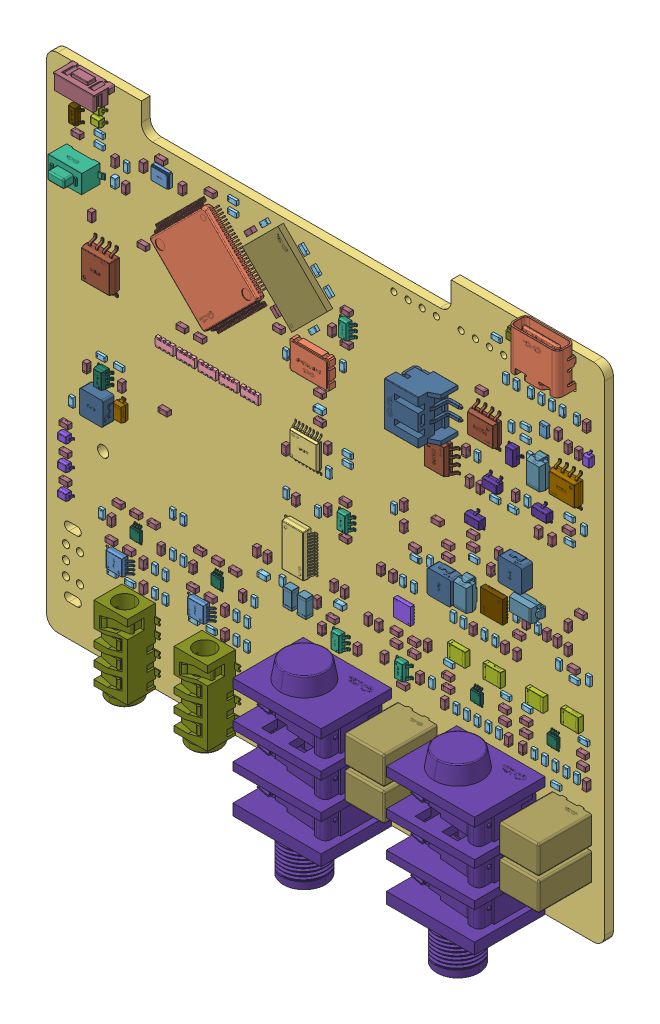
SolidWorks assembly 3D_board_2024-11-06, configuration 默认. Lengths in mm. (continued)
Components (placement in the parent): (continued)
- 3D_board_2024-11-06.step-1: 3D_board_2024-11-06.step [默认] at origin size (99.97 100.01 16.2) (continued)
  - iqks-C60.step-1: iqks-C60.step [默认] at (54.2011 -13.843 1.5862) x (-1 0 0) z (0 0 1) size (1.6 0.8 0.8) (continued)
    - C0603.step-1: C0603.step [默认] at origin size (1.6 0.8 0.8)
      - SOLID-10.step-1: SOLID-10.step [默认] at origin size (1.6 0.8 0.8)
  - iqks-C64.step-1: iqks-C64.step [默认] at (64.3026 -66.7617 1.5862) size (1.6 0.8 0.8)
    - C0603.step-1: C0603.step [默认] at origin size (1.6 0.8 0.8)
      - SOLID-10.step-1: SOLID-10.step [默认] at origin size (1.6 0.8 0.8)
  - iqks-C150.step-1: iqks-C150.step [默认] at (51.6811 -62.7701 1.5862) size (1.6 0.8 0.8)
    - C0603.step-1: C0603.step [默认] at origin size (1.6 0.8 0.8)
      - SOLID-10.step-1: SOLID-10.step [默认] at origin size (1.6 0.8 0.8)
  - iqks-C153.step-1: iqks-C153.step [默认] at (80.0102 -41.0211 1.5862) x (0 -1 0) z (0 0 1) size (1.6 0.8 0.8)
    - C0603.step-1: C0603.step [默认] at origin size (1.6 0.8 0.8)
      - SOLID-10.step-1: SOLID-10.step [默认] at origin size (1.6 0.8 0.8)
  - iqks-C15.step-1: iqks-C15.step [默认] at (71.7551 -65.8101 1.5862) x (0 1 0) z (0 0 1) size (1.6 0.8 0.8)
    - C0603.step-1: C0603.step [默认] at origin size (1.6 0.8 0.8)
      - SOLID-10.step-1: SOLID-10.step [默认] at origin size (1.6 0.8 0.8)
  - iqks-C16.step-1: iqks-C16.step [默认] at (83.1852 -65.8101 1.5862) x (0 1 0) z (0 0 1) size (1.6 0.8 0.8)
    - C0603.step-1: C0603.step [默认] at origin size (1.6 0.8 0.8)
      - SOLID-10.step-1: SOLID-10.step [默认] at origin size (1.6 0.8 0.8)
  - iqks-C38.step-1: iqks-C38.step [默认] at (85.7252 -65.8101 1.5862) x (0 1 0) z (0 0 1) size (1.6 0.8 0.8)
    - C0603.step-1: C0603.step [默认] at origin size (1.6 0.8 0.8)
      - SOLID-10.step-1: SOLID-10.step [默认] at origin size (1.6 0.8 0.8)
  - iqks-C39.step-1: iqks-C39.step [默认] at (97.1552 -65.8101 1.5862) x (0 1 0) z (0 0 1) size (1.6 0.8 0.8)
    - C0603.step-1: C0603.step [默认] at origin size (1.6 0.8 0.8)
      - SOLID-10.step-1: SOLID-10.step [默认] at origin size (1.6 0.8 0.8)
  - iqks-C17.step-1: iqks-C17.step [默认] at (26.6701 -67.3101 1.5862) x (0 -1 0) z (0 0 1) size (1.6 0.8 0.8)
    - C0603.step-1: C0603.step [默认] at origin size (1.6 0.8 0.8)
      - SOLID-10.step-1: SOLID-10.step [默认] at origin size (1.6 0.8 0.8)
  - iqks-C18.step-1: iqks-C18.step [默认] at (35.5601 -67.3101 1.5862) x (0 -1 0) z (0 0 1) size (1.6 0.8 0.8)
    - C0603.step-1: C0603.step [默认] at origin size (1.6 0.8 0.8)
      - SOLID-10.step-1: SOLID-10.step [默认] at origin size (1.6 0.8 0.8)
  - iqks-C50.step-1: iqks-C50.step [默认] at (12.065 -67.3101 1.5862) x (0 -1 0) z (0 0 1) size (1.6 0.8 0.8)
    - C0603.step-1: C0603.step [默认] at origin size (1.6 0.8 0.8)
      - SOLID-10.step-1: SOLID-10.step [默认] at origin size (1.6 0.8 0.8)
  - iqks-C51.step-1: iqks-C51.step [默认] at (20.955 -67.3101 1.5862) x (0 -1 0) z (0 0 1) size (1.6 0.8 0.8)
    - C0603.step-1: C0603.step [默认] at origin size (1.6 0.8 0.8)
      - SOLID-10.step-1: SOLID-10.step [默认] at origin size (1.6 0.8 0.8)
  - iqks-C22.step-1: iqks-C22.step [默认] at (17.78 -74.9301 1.5862) x (0 1 0) z (0 0 1) size (1.6 0.8 0.8)
    - C0603.step-1: C0603.step [默认] at origin size (1.6 0.8 0.8)
      - SOLID-10.step-1: SOLID-10.step [默认] at origin size (1.6 0.8 0.8)
  - iqks-C28.step-1: iqks-C28.step [默认] at (17.78 -71.1201 1.5862) x (0 -1 0) z (0 0 1) size (1.6 0.8 0.8)
    - C0603.step-1: C0603.step [默认] at origin size (1.6 0.8 0.8)
      - SOLID-10.step-1: SOLID-10.step [默认] at origin size (1.6 0.8 0.8)
  - iqks-C31.step-1: iqks-C31.step [默认] at (32.3851 -74.9301 1.5862) x (0 1 0) z (0 0 1) size (1.6 0.8 0.8)
    - C0603.step-1: C0603.step [默认] at origin size (1.6 0.8 0.8)
      - SOLID-10.step-1: SOLID-10.step [默认] at origin size (1.6 0.8 0.8)
  - iqks-C32.step-1: iqks-C32.step [默认] at (32.3851 -71.1201 1.5862) x (0 -1 0) z (0 0 1) size (1.6 0.8 0.8)
    - C0603.step-1: C0603.step [默认] at origin size (1.6 0.8 0.8)
      - SOLID-10.step-1: SOLID-10.step [默认] at origin size (1.6 0.8 0.8)
  - iqks-C113.step-1: iqks-C113.step [默认] at (53.8401 -57.5551 1.5862) x (0 1 0) z (0 0 1) size (1.6 0.8 0.8)
    - C0603.step-1: C0603.step [默认] at origin size (1.6 0.8 0.8)
      - SOLID-10.step-1: SOLID-10.step [默认] at origin size (1.6 0.8 0.8)
  - iqks-C116.step-1: iqks-C116.step [默认] at (38.1001 -59.0551 1.5862) x (0 1 0) z (0 0 1) size (1.6 0.8 0.8)
    - C0603.step-1: C0603.step [默认] at origin size (1.6 0.8 0.8)
      - SOLID-10.step-1: SOLID-10.step [默认] at origin size (1.6 0.8 0.8)
  - iqks-C25.step-1: iqks-C25.step [默认] at (63.1191 -60.9601 1.5862) x (-1 0 0) z (0 0 1) size (1.6 0.8 0.8)
    - C0603.step-1: C0603.step [默认] at origin size (1.6 0.8 0.8)
      - SOLID-10.step-1: SOLID-10.step [默认] at origin size (1.6 0.8 0.8)
  - iqks-C27.step-1: iqks-C27.step [默认] at (66.2941 -60.9601 1.5862) x (-1 0 0) z (0 0 1) size (1.6 0.8 0.8)
    - C0603.step-1: C0603.step [默认] at origin size (1.6 0.8 0.8)
      - SOLID-10.step-1: SOLID-10.step [默认] at origin size (1.6 0.8 0.8)
  - iqks-C129.step-1: iqks-C129.step [默认] at (58.0391 -59.6901 1.5862) x (0 1 0) z (0 0 1) size (1.6 0.8 0.8)
    - C0603.step-1: C0603.step [默认] at origin size (1.6 0.8 0.8)
      - SOLID-10.step-1: SOLID-10.step [默认] at origin size (1.6 0.8 0.8)
  - iqks-C154.step-1: iqks-C154.step [默认] at (60.3251 -50.8001 1.5862) x (0 -1 0) z (0 0 1) size (1.6 0.8 0.8)
    - C0603.step-1: C0603.step [默认] at origin size (1.6 0.8 0.8)
      - SOLID-10.step-1: SOLID-10.step [默认] at origin size (1.6 0.8 0.8)
  - iqks-C138.step-1: iqks-C138.step [默认] at (85.0902 -48.6411 1.5862) size (1.6 0.8 0.8)
    - C0603.step-1: C0603.step [默认] at origin size (1.6 0.8 0.8)
      - SOLID-10.step-1: SOLID-10.step [默认] at origin size (1.6 0.8 0.8)
  - iqks-C139.step-1: iqks-C139.step [默认] at (84.7092 -51.8161 1.5862) x (0 1 0) z (0 0 1) size (1.6 0.8 0.8)
    - C0603.step-1: C0603.step [默认] at origin size (1.6 0.8 0.8)
      - SOLID-10.step-1: SOLID-10.step [默认] at origin size (1.6 0.8 0.8)
  - iqks-C149.step-1: iqks-C149.step [默认] at (82.5502 -51.8161 1.5862) x (0 1 0) z (0 0 1) size (1.6 0.8 0.8)
    - C0603.step-1: C0603.step [默认] at origin size (1.6 0.8 0.8)
      - SOLID-10.step-1: SOLID-10.step [默认] at origin size (1.6 0.8 0.8)
  - iqks-C3.step-1: iqks-C3.step [默认] at (16.51 -64.1351 1.5862) x (-1 0 0) z (0 0 1) size (1.6 0.8 0.8)
    - C0603.step-1: C0603.step [默认] at origin size (1.6 0.8 0.8)
      - SOLID-10.step-1: SOLID-10.step [默认] at origin size (1.6 0.8 0.8)
  - iqks-C4.step-1: iqks-C4.step [默认] at (19.62 -64.1351 1.5862) size (1.6 0.8 0.8)
    - C0603.step-1: C0603.step [默认] at origin size (1.6 0.8 0.8)
      - SOLID-10.step-1: SOLID-10.step [默认] at origin size (1.6 0.8 0.8)
  - iqks-C5.step-1: iqks-C5.step [默认] at (13.335 -64.1351 1.5862) size (1.6 0.8 0.8)
    - C0603.step-1: C0603.step [默认] at origin size (1.6 0.8 0.8)
      - SOLID-10.step-1: SOLID-10.step [默认] at origin size (1.6 0.8 0.8)
  - iqks-C19.step-1: iqks-C19.step [默认] at (31.1151 -64.1351 1.5862) x (-1 0 0) z (0 0 1) size (1.6 0.8 0.8)
    - C0603.step-1: C0603.step [默认] at origin size (1.6 0.8 0.8)
      - SOLID-10.step-1: SOLID-10.step [默认] at origin size (1.6 0.8 0.8)
  - iqks-C20.step-1: iqks-C20.step [默认] at (34.225 -64.1351 1.5862) size (1.6 0.8 0.8)
    - C0603.step-1: C0603.step [默认] at origin size (1.6 0.8 0.8)
      - SOLID-10.step-1: SOLID-10.step [默认] at origin size (1.6 0.8 0.8)
  - iqks-C21.step-1: iqks-C21.step [默认] at (27.9401 -64.1351 1.5862) size (1.6 0.8 0.8)
    - C0603.step-1: C0603.step [默认] at origin size (1.6 0.8 0.8)
      - SOLID-10.step-1: SOLID-10.step [默认] at origin size (1.6 0.8 0.8)
  - iqks-C29.step-1: iqks-C29.step [默认] at (12.065 -70.4851 1.5862) size (1.6 0.8 0.8)
    - C0603.step-1: C0603.step [默认] at origin size (1.6 0.8 0.8)
      - SOLID-10.step-1: SOLID-10.step [默认] at origin size (1.6 0.8 0.8)
  - iqks-C30.step-1: iqks-C30.step [默认] at (15.24 -70.4851 1.5862) x (-1 0 0) z (0 0 1) size (1.6 0.8 0.8)
    - C0603.step-1: C0603.step [默认] at origin size (1.6 0.8 0.8)
      - SOLID-10.step-1: SOLID-10.step [默认] at origin size (1.6 0.8 0.8)
  - iqks-C33.step-1: iqks-C33.step [默认] at (26.6701 -70.4851 1.5862) size (1.6 0.8 0.8)
    - C0603.step-1: C0603.step [默认] at origin size (1.6 0.8 0.8)
      - SOLID-10.step-1: SOLID-10.step [默认] at origin size (1.6 0.8 0.8)
  - iqks-C36.step-1: iqks-C36.step [默认] at (29.8451 -70.4851 1.5862) x (-1 0 0) z (0 0 1) size (1.6 0.8 0.8)
    - C0603.step-1: C0603.step [默认] at origin size (1.6 0.8 0.8)
      - SOLID-10.step-1: SOLID-10.step [默认] at origin size (1.6 0.8 0.8)
  - iqks-C42.step-1: iqks-C42.step [默认] at (76.2002 -29.2101 1.5862) x (0 1 0) z (0 0 1) size (1.6 0.8 0.8)
    - C0603.step-1: C0603.step [默认] at origin size (1.6 0.8 0.8)
      - SOLID-10.step-1: SOLID-10.step [默认] at origin size (1.6 0.8 0.8)
  - iqks-C43.step-1: iqks-C43.step [默认] at (92.0752 -13.97 1.5862) x (0 1 0) z (0 0 1) size (1.6 0.8 0.8)
    - C0603.step-1: C0603.step [默认] at origin size (1.6 0.8 0.8)
      - SOLID-10.step-1: SOLID-10.step [默认] at origin size (1.6 0.8 0.8)
  - iqks-C44.step-1: iqks-C44.step [默认] at (93.8532 -15.113 1.5862) x (0 -1 0) z (0 0 1) size (1.6 0.8 0.8)
    - C0603.step-1: C0603.step [默认] at origin size (1.6 0.8 0.8)
      - SOLID-10.step-1: SOLID-10.step [默认] at origin size (1.6 0.8 0.8)
  - iqks-C46.step-1: iqks-C46.step [默认] at (78.1052 -29.2101 1.5862) x (0 1 0) z (0 0 1) size (1.6 0.8 0.8)
    - C0603.step-1: C0603.step [默认] at origin size (1.6 0.8 0.8)
      - SOLID-10.step-1: SOLID-10.step [默认] at origin size (1.6 0.8 0.8)
  - iqks-C49.step-1: iqks-C49.step [默认] at (93.9802 -27.9401 1.5862) x (-1 0 0) z (0 0 1) size (1.6 0.8 0.8)
    - C0603.step-1: C0603.step [默认] at origin size (1.6 0.8 0.8)
      - SOLID-10.step-1: SOLID-10.step [默认] at origin size (1.6 0.8 0.8)
  - iqks-C54.step-1: iqks-C54.step [默认] at (81.4072 -37.8461 1.5862) x (0 1 0) z (0 0 1) size (1.6 0.8 0.8)
    - C0603.step-1: C0603.step [默认] at origin size (1.6 0.8 0.8)
      - SOLID-10.step-1: SOLID-10.step [默认] at origin size (1.6 0.8 0.8)
  - iqks-C56.step-1: iqks-C56.step [默认] at (76.8352 -37.2111 1.5862) x (-1 0 0) z (0 0 1) size (1.6 0.8 0.8)
    - C0603.step-1: C0603.step [默认] at origin size (1.6 0.8 0.8)
      - SOLID-10.step-1: SOLID-10.step [默认] at origin size (1.6 0.8 0.8)
  - iqks-C61.step-1: iqks-C61.step [默认] at (56.1101 -65.3101 1.5862) x (0 1 0) z (0 0 1) size (1.6 0.8 0.8)
    - C0603.step-1: C0603.step [默认] at origin size (1.6 0.8 0.8)
      - SOLID-10.step-1: SOLID-10.step [默认] at origin size (1.6 0.8 0.8)
  - iqks-C134.step-1: iqks-C134.step [默认] at (75.5652 -24.765 1.5862) x (0 -1 0) z (0 0 1) size (1.6 0.8 0.8)
    - C0603.step-1: C0603.step [默认] at origin size (1.6 0.8 0.8)
      - SOLID-10.step-1: SOLID-10.step [默认] at origin size (1.6 0.8 0.8)
  - iqks-C135.step-1: iqks-C135.step [默认] at (84.4552 -27.3051 1.5862) x (0 -1 0) z (0 0 1) size (1.6 0.8 0.8)
    - C0603.step-1: C0603.step [默认] at origin size (1.6 0.8 0.8)
      - SOLID-10.step-1: SOLID-10.step [默认] at origin size (1.6 0.8 0.8)
  - iqks-C140.step-1: iqks-C140.step [默认] at (72.3901 -42.9261 1.5862) x (-1 0 0) z (0 0 1) size (1.6 0.8 0.8)
    - C0603.step-1: C0603.step [默认] at origin size (1.6 0.8 0.8)
      - SOLID-10.step-1: SOLID-10.step [默认] at origin size (1.6 0.8 0.8)
  - iqks-C141.step-1: iqks-C141.step [默认] at (72.3901 -41.0211 1.5862) x (-1 0 0) z (0 0 1) size (1.6 0.8 0.8)
    - C0603.step-1: C0603.step [默认] at origin size (1.6 0.8 0.8)
      - SOLID-10.step-1: SOLID-10.step [默认] at origin size (1.6 0.8 0.8)
  - iqks-C146.step-1: iqks-C146.step [默认] at (90.0432 -46.1011 1.5862) x (0 -1 0) z (0 0 1) size (1.6 0.8 0.8)
    - C0603.step-1: C0603.step [默认] at origin size (1.6 0.8 0.8)
      - SOLID-10.step-1: SOLID-10.step [默认] at origin size (1.6 0.8 0.8)
  - iqks-C147.step-1: iqks-C147.step [默认] at (91.9482 -46.1011 1.5862) x (0 1 0) z (0 0 1) size (1.6 0.8 0.8)
    - C0603.step-1: C0603.step [默认] at origin size (1.6 0.8 0.8)
      - SOLID-10.step-1: SOLID-10.step [默认] at origin size (1.6 0.8 0.8)
  - iqks-C151.step-1: iqks-C151.step [默认] at (49.7601 -65.3101 1.5862) x (0 -1 0) z (0 0 1) size (1.6 0.8 0.8)
    - C0603.step-1: C0603.step [默认] at origin size (1.6 0.8 0.8)
      - SOLID-10.step-1: SOLID-10.step [默认] at origin size (1.6 0.8 0.8)
  - iqks-C156.step-1: iqks-C156.step [默认] at (64.4229 -42.0779 1.5862) x (0 -1 0) z (0 0 1) size (1.6 0.8 0.8)
    - C0603.step-1: C0603.step [默认] at origin size (1.6 0.8 0.8)
      - SOLID-10.step-1: SOLID-10.step [默认] at origin size (1.6 0.8 0.8)
  - iqks-C159.step-1: iqks-C159.step [默认] at (93.8532 -46.4821 1.5862) x (0 -1 0) z (0 0 1) size (1.6 0.8 0.8)
    - C0603.step-1: C0603.step [默认] at origin size (1.6 0.8 0.8)
      - SOLID-10.step-1: SOLID-10.step [默认] at origin size (1.6 0.8 0.8)
  - iqks-C162.step-1: iqks-C162.step [默认] at (93.8532 -42.7991 1.5862) x (0 -1 0) z (0 0 1) size (1.6 0.8 0.8)
    - C0603.step-1: C0603.step [默认] at origin size (1.6 0.8 0.8)
      - SOLID-10.step-1: SOLID-10.step [默认] at origin size (1.6 0.8 0.8)
  - iqks-C163.step-1: iqks-C163.step [默认] at (64.4229 -38.7759 1.5862) x (0 -1 0) z (0 0 1) size (1.6 0.8 0.8)
    - C0603.step-1: C0603.step [默认] at origin size (1.6 0.8 0.8)
      - SOLID-10.step-1: SOLID-10.step [默认] at origin size (1.6 0.8 0.8)
  - iqks-C1.step-1: iqks-C1.step [默认] at (54.2011 -18.923 1.5862) size (1.6 0.8 0.8)
    - C0603.step-1: C0603.step [默认] at origin size (1.6 0.8 0.8)
      - SOLID-10.step-1: SOLID-10.step [默认] at origin size (1.6 0.8 0.8)
  - iqks-C2.step-1: iqks-C2.step [默认] at (51.5621 -18.0991 1.5862) x (0 1 0) z (0 0 1) size (1.6 0.8 0.8)
    - C0603.step-1: C0603.step [默认] at origin size (1.6 0.8 0.8)
      - SOLID-10.step-1: SOLID-10.step [默认] at origin size (1.6 0.8 0.8)
  - iqks-C57.step-1: iqks-C57.step [默认] at (86.3602 -46.1011 1.5862) x (0 -1 0) z (0 0 1) size (1.6 0.8 0.8)
    - C0603.step-1: C0603.step [默认] at origin size (1.6 0.8 0.8)
      - SOLID-10.step-1: SOLID-10.step [默认] at origin size (1.6 0.8 0.8)
  - iqks-C94.step-1: iqks-C94.step [默认] at (53.9751 -49.1491 1.5862) size (1.6 0.8 0.8)
    - C0603.step-1: C0603.step [默认] at origin size (1.6 0.8 0.8)
      - SOLID-10.step-1: SOLID-10.step [默认] at origin size (1.6 0.8 0.8)
  - iqks-C95.step-1: iqks-C95.step [默认] at (50.8001 -46.3551 1.5862) x (0 -1 0) z (0 0 1) size (1.6 0.8 0.8)
    - C0603.step-1: C0603.step [默认] at origin size (1.6 0.8 0.8)
      - SOLID-10.step-1: SOLID-10.step [默认] at origin size (1.6 0.8 0.8)
  - iqks-C96.step-1: iqks-C96.step [默认] at (60.9601 -64.1351 1.5862) x (0 1 0) z (0 0 1) size (1.6 0.8 0.8)
    - C0603.step-1: C0603.step [默认] at origin size (1.6 0.8 0.8)
      - SOLID-10.step-1: SOLID-10.step [默认] at origin size (1.6 0.8 0.8)
  - iqks-C97.step-1: iqks-C97.step [默认] at (67.3101 -64.1351 1.5862) x (0 1 0) z (0 0 1) size (1.6 0.8 0.8)
    - C0603.step-1: C0603.step [默认] at origin size (1.6 0.8 0.8)
      - SOLID-10.step-1: SOLID-10.step [默认] at origin size (1.6 0.8 0.8)
  - iqks-C148.step-1: iqks-C148.step [默认] at (76.8352 -51.8161 1.5862) x (0 -1 0) z (0 0 1) size (1.6 0.8 0.8)
    - C0603.step-1: C0603.step [默认] at origin size (1.6 0.8 0.8)
      - SOLID-10.step-1: SOLID-10.step [默认] at origin size (1.6 0.8 0.8)
  - iqks-C164.step-1: iqks-C164.step [默认] at (66.4211 -44.4501 1.5862) x (-1 0 0) z (0 0 1) size (1.6 0.8 0.8)
    - C0603.step-1: C0603.step [默认] at origin size (1.6 0.8 0.8)
      - SOLID-10.step-1: SOLID-10.step [默认] at origin size (1.6 0.8 0.8)
  - iqks-C165.step-1: iqks-C165.step [默认] at (94.8692 -49.0221 1.5862) x (-1 0 0) z (0 0 1) size (1.6 0.8 0.8)
    - C0603.step-1: C0603.step [默认] at origin size (1.6 0.8 0.8)
      - SOLID-10.step-1: SOLID-10.step [默认] at origin size (1.6 0.8 0.8)
  - iqks-C166.step-1: iqks-C166.step [默认] at (70.4851 -38.2271 1.5862) x (-1 0 0) z (0 0 1) size (1.6 0.8 0.8)
    - C0603.step-1: C0603.step [默认] at origin size (1.6 0.8 0.8)
      - SOLID-10.step-1: SOLID-10.step [默认] at origin size (1.6 0.8 0.8)
  - iqks-C167.step-1: iqks-C167.step [默认] at (96.1392 -39.8781 1.5862) size (1.6 0.8 0.8)
    - C0603.step-1: C0603.step [默认] at origin size (1.6 0.8 0.8)
      - SOLID-10.step-1: SOLID-10.step [默认] at origin size (1.6 0.8 0.8)
  - iqks-C168.step-1: iqks-C168.step [默认] at (49.4103 -33.4035 1.5862) size (1.6 0.8 0.8)
    - C0603.step-1: C0603.step [默认] at origin size (1.6 0.8 0.8)
      - SOLID-10.step-1: SOLID-10.step [默认] at origin size (1.6 0.8 0.8)
  - iqks-C169.step-1: iqks-C169.step [默认] at (90.9728 -30.8843 1.5862) x (0 1 0) z (0 0 1) size (1.6 0.8 0.8)
    - C0603.step-1: C0603.step [默认] at origin size (1.6 0.8 0.8)
      - SOLID-10.step-1: SOLID-10.step [默认] at origin size (1.6 0.8 0.8)
  - iqks-C173.step-1: iqks-C173.step [默认] at (78.3514 -14.0943 1.5862) x (-1 0 0) z (0 0 1) size (1.6 0.8 0.8)
    - C0603.step-1: C0603.step [默认] at origin size (1.6 0.8 0.8)
      - SOLID-10.step-1: SOLID-10.step [默认] at origin size (1.6 0.8 0.8)
  - iqks-C174.step-1: iqks-C174.step [默认] at (5.969 -10.414 1.5862) size (1.6 0.8 0.8)
    - C0603.step-1: C0603.step [默认] at origin size (1.6 0.8 0.8)
      - SOLID-10.step-1: SOLID-10.step [默认] at origin size (1.6 0.8 0.8)
  - iqks-C9.step-1: iqks-C9.step [默认] at (71.3741 -84.1142 1.5862) x (-1 0 0) z (0 0 1) size (1.6 0.8 0.8)
    - C0603.step-1: C0603.step [默认] at origin size (1.6 0.8 0.8)
      - SOLID-10.step-1: SOLID-10.step [默认] at origin size (1.6 0.8 0.8)
  - iqks-C52.step-1: iqks-C52.step [默认] at (64.0081 -84.1142 1.5862) size (1.6 0.8 0.8)
    - C0603.step-1: C0603.step [默认] at origin size (1.6 0.8 0.8)
      - SOLID-10.step-1: SOLID-10.step [默认] at origin size (1.6 0.8 0.8)
  - iqks-C115.step-1: iqks-C115.step [默认] at (48.8951 -61.5951 1.5862) x (0 -1 0) z (0 0 1) size (1.6 0.8 0.8)
    - C0603.step-1: C0603.step [默认] at origin size (1.6 0.8 0.8)
      - SOLID-10.step-1: SOLID-10.step [默认] at origin size (1.6 0.8 0.8)
  - iqks-D2.step-1: iqks-D2.step [默认] at (86.9952 -42.9261 1.5862) x (-1 0 0) z (0 0 1) size (5.21 2.62 2.16)
    - SMA_L4.2-W2.6-LS5.3-RD.step-1: SMA_L4.2-W2.6-LS5.3-RD.step [默认] at origin size (5.21 2.62 2.16)
      - COMPOUND-11.step-1: COMPOUND-11.step [默认] at origin size (5.21 2.62 2.16)
  - iqks-D3.step-1: iqks-D3.step [默认] at (76.2002 -46.3551 1.5862) x (0 1 0) z (0 0 1) size (5.21 2.62 2.16)
    - SMA_L4.2-W2.6-LS5.3-RD.step-1: SMA_L4.2-W2.6-LS5.3-RD.step [默认] at origin size (5.21 2.62 2.16)
      - COMPOUND-11.step-1: COMPOUND-11.step [默认] at origin size (5.21 2.62 2.16)
  - iqks-D1.step-1: iqks-D1.step [默认] at (89.2812 -20.955 1.5862) x (0 1 0) z (0 0 1) size (5.21 2.62 2.16)
    - SMA_L4.2-W2.6-LS5.3-RD.step-1: SMA_L4.2-W2.6-LS5.3-RD.step [默认] at origin size (5.21 2.62 2.16)
      - COMPOUND-11.step-1: COMPOUND-11.step [默认] at origin size (5.21 2.62 2.16)
  - iqks-U17.step-1: iqks-U17.step [默认] at (10.7362 -45.5718 1.5862) size (2.81 2.9 1.65)
    - SOT-23-6_L2.9-W1.6-P0.95-LS2.8-BR.step-1: SOT-23-6_L2.9-W1.6-P0.95-LS2.8-BR.step [默认] at origin size (2.81 2.9 1.65)
      - COMPOUND-12.step-1: COMPOUND-12.step [默认] at origin size (2.81 2.9 1.65)
  - iqks-J4.step-1: iqks-J4.step [默认] at (30.8651 -83.1852 1.5862) size (7.9 14.5 5.75)
    - AUDIO-SMD_PJ-393.step-1: AUDIO-SMD_PJ-393.step [默认] at origin size (7.9 14.5 5.75)
      - COMPOUND-13.step-1: COMPOUND-13.step [默认] at origin size (7.9 14.5 5.75)
  - iqks-J5.step-1: iqks-J5.step [默认] at (16.51 -83.1852 1.5862) size (7.9 14.5 5.75)
    - AUDIO-SMD_PJ-393.step-1: AUDIO-SMD_PJ-393.step [默认] at origin size (7.9 14.5 5.75)
      - COMPOUND-13.step-1: COMPOUND-13.step [默认] at origin size (7.9 14.5 5.75)
  - iqks-Q6.step-1: iqks-Q6.step [默认] at (84.2012 -20.955 1.5862) x (0 1 0) z (0 0 1) size (2.8 2.7 1.35)
    - SOT-23-3_L2.9-W1.6-P1.90-LS2.8-BR.step-1: SOT-23-3_L2.9-W1.6-P1.90-LS2.8-BR.step [默认] at origin size (2.8 2.7 1.35)
      - SOLID-14.step-1: SOLID-14.step [默认] at origin size (2.8 2.7 1.35)
  - iqks-Q7.step-1: iqks-Q7.step [默认] at (89.5352 -27.3051 1.5862) x (-1 0 0) z (0 0 1) size (2.8 2.7 1.35)
    - SOT-23-3_L2.9-W1.6-P1.90-LS2.8-BR.step-1: SOT-23-3_L2.9-W1.6-P1.90-LS2.8-BR.step [默认] at origin size (2.8 2.7 1.35)
      - SOLID-14.step-1: SOLID-14.step [默认] at origin size (2.8 2.7 1.35)
  - iqks-Q8.step-1: iqks-Q8.step [默认] at (80.6452 -27.3051 1.5862) size (2.8 2.7 1.35)
    - SOT-23-3_L2.9-W1.6-P1.90-LS2.8-BR.step-1: SOT-23-3_L2.9-W1.6-P1.90-LS2.8-BR.step [默认] at origin size (2.8 2.7 1.35)
      - SOLID-14.step-1: SOLID-14.step [默认] at origin size (2.8 2.7 1.35)
  - iqks-Q5.step-1: iqks-Q5.step [默认] at (77.4702 -34.4171 1.5862) x (-1 0 0) z (0 0 1) size (2.8 2.7 1.35)
    - SOT-23-3_L2.9-W1.6-P1.90-LS2.8-BR.step-1: SOT-23-3_L2.9-W1.6-P1.90-LS2.8-BR.step [默认] at origin size (2.8 2.7 1.35)
      - SOLID-14.step-1: SOLID-14.step [默认] at origin size (2.8 2.7 1.35)
  - iqks-U27.step-1: iqks-U27.step [默认] at (80.6452 -46.1011 1.5862) x (0 -1 0) z (0 0 1) size (4.02 4.02 0.92)
    - QFN-24_L4.0-W4.0-P0.50-TL-EP2.6.step-1: QFN-24_L4.0-W4.0-P0.50-TL-EP2.6.step [默认] at origin size (4.02 4.02 0.92)
      - SOLID-15.step-1: SOLID-15.step [默认] at origin size (4.02 4.02 0.92)
  - iqks-L4.step-1: iqks-L4.step [默认] at (89.5352 -14.605 1.5862) x (0 1 0) z (0 0 1) size (2 1.3 0.61)
    - L0805.step-1: L0805.step [默认] at origin size (2 1.3 0.61)
      - COMPOUND-16.step-1: COMPOUND-16.step [默认] at origin size (2 1.3 0.61)
  - iqks-J3.step-1: iqks-J3.step [默认] at (90.1702 -3.81 1.5862) x (-1 0 0) z (0 0 1) size (8.94 7.9 4.1)
    - usb-c_smd-type-c-31-m-12.step-1: usb-c_smd-type-c-31-m-12.step [默认] at origin size (8.94 7.9 4.1)
      - COMPOUND-17.step-1: COMPOUND-17.step [默认] at origin size (8.94 7.9 4.1)
  - iqks-U15.step-1: iqks-U15.step [默认] at (46.9901 -38.7351 1.5862) size (5 6.41 1.05)
    - TSSOP-16_L5.0-W4.4-P0.65-LS6.4-BL.step-1: TSSOP-16_L5.0-W4.4-P0.65-LS6.4-BL.step [默认] at origin size (5 6.41 1.05)
      - COMPOUND-18.step-1: COMPOUND-18.step [默认] at origin size (5 6.41 1.05)
  - iqks-LED3.step-1: iqks-LED3.step [默认] at (52.7051 -80.7722 0) x (1 0 0) z (0 0 -1) size (2.01 1.25 1)
    - LED_0805.step-1: LED_0805.step [默认] at origin size (2.01 1.25 1)
      - COMPOUND-19.step-1: COMPOUND-19.step [默认] at origin size (2.01 1.25 1)
  - iqks-LED2.step-1: iqks-LED2.step [默认] at (80.8992 -80.7722 0) x (1 0 0) z (0 0 -1) size (2.01 1.25 1)
    - LED_0805.step-1: LED_0805.step [默认] at origin size (2.01 1.25 1)
      - COMPOUND-19.step-1: COMPOUND-19.step [默认] at origin size (2.01 1.25 1)
  - iqks-L9.step-1: iqks-L9.step [默认] at (49.4103 -31.4985 1.5862) size (1.62 0.82 0.82)
    - BEAD-SMD_L1.6-W0.8-P1.6.step-1: BEAD-SMD_L1.6-W0.8-P1.6.step [默认] at origin size (1.62 0.82 0.82)
      - SOLID-20.step-1: SOLID-20.step [默认] at origin size (1.62 0.82 0.82)
  - iqks-L10.step-1: iqks-L10.step [默认] at (53.0081 -60.0001 1.5862) size (1.62 0.82 0.82)
    - BEAD-SMD_L1.6-W0.8-P1.6.step-1: BEAD-SMD_L1.6-W0.8-P1.6.step [默认] at origin size (1.62 0.82 0.82)
      - SOLID-20.step-1: SOLID-20.step [默认] at origin size (1.62 0.82 0.82)
  - iqks-L11.step-1: iqks-L11.step [默认] at (39.3701 -62.2301 1.5862) x (-1 0 0) z (0 0 1) size (1.62 0.82 0.82)
    - BEAD-SMD_L1.6-W0.8-P1.6.step-1: BEAD-SMD_L1.6-W0.8-P1.6.step [默认] at origin size (1.62 0.82 0.82)
      - SOLID-20.step-1: SOLID-20.step [默认] at origin size (1.62 0.82 0.82)
  - iqks-L6.step-1: iqks-L6.step [默认] at (12.7 -14.478 1.5862) x (0 -1 0) z (0 0 1) size (1.62 0.82 0.82)
    - BEAD-SMD_L1.6-W0.8-P1.6.step-1: BEAD-SMD_L1.6-W0.8-P1.6.step [默认] at origin size (1.62 0.82 0.82)
      - SOLID-20.step-1: SOLID-20.step [默认] at origin size (1.62 0.82 0.82)
  - iqks-LDO1.step-1: iqks-LDO1.step [默认] at (54.2011 -16.383 1.5862) x (0 1 0) z (0 0 1) size (2.9 3.01 1.25)
    - SOT-23-5_L3.0-W1.7-P0.95-LS2.8-BL.step-1: SOT-23-5_L3.0-W1.7-P0.95-LS2.8-BL.step [默认] at origin size (2.9 3.01 1.25)
      - COMPOUND-21.step-1: COMPOUND-21.step [默认] at origin size (2.9 3.01 1.25)
  - iqks-LDO2.step-1: iqks-LDO2.step [默认] at (53.9751 -46.3551 1.5862) x (0 1 0) z (0 0 1) size (2.9 3.01 1.25)
    - SOT-23-5_L3.0-W1.7-P0.95-LS2.8-BL.step-1: SOT-23-5_L3.0-W1.7-P0.95-LS2.8-BL.step [默认] at origin size (2.9 3.01 1.25)
      - COMPOUND-21.step-1: COMPOUND-21.step [默认] at origin size (2.9 3.01 1.25)
  - iqks-LDO3.step-1: iqks-LDO3.step [默认] at (64.3026 -64.2217 1.5862) x (0 -1 0) z (0 0 1) size (2.9 3.01 1.25)
    - SOT-23-5_L3.0-W1.7-P0.95-LS2.8-BL.step-1: SOT-23-5_L3.0-W1.7-P0.95-LS2.8-BL.step [默认] at origin size (2.9 3.01 1.25)
      - COMPOUND-21.step-1: COMPOUND-21.step [默认] at origin size (2.9 3.01 1.25)
  - iqks-U28.step-1: iqks-U28.step [默认] at (52.9351 -65.4371 1.5862) x (0 1 0) z (0 0 1) size (2.9 3.01 1.25)
    - SOT-23-5_L3.0-W1.7-P0.95-LS2.8-BL.step-1: SOT-23-5_L3.0-W1.7-P0.95-LS2.8-BL.step [默认] at origin size (2.9 3.01 1.25)
      - COMPOUND-21.step-1: COMPOUND-21.step [默认] at origin size (2.9 3.01 1.25)
  - iqks-D10.step-1: iqks-D10.step [默认] at (9.779 -4.445 1.5862) size (2.51 1.3 1.2)
    - SOD-323_L1.8-W1.3-LS2.5-RD.step-1: SOD-323_L1.8-W1.3-LS2.5-RD.step [默认] at origin size (2.51 1.3 1.2)
      - COMPOUND-22.step-1: COMPOUND-22.step [默认] at origin size (2.51 1.3 1.2)
  - iqks-D9.step-1: iqks-D9.step [默认] at (9.779 -6.35 1.5862) size (2.51 1.3 1.2)
    - SOD-323_L1.8-W1.3-LS2.5-RD.step-1: SOD-323_L1.8-W1.3-LS2.5-RD.step [默认] at origin size (2.51 1.3 1.2)
      - COMPOUND-22.step-1: COMPOUND-22.step [默认] at origin size (2.51 1.3 1.2)
  - iqks-U5.step-1: iqks-U5.step [默认] at (64.3891 -55.2451 1.5862) x (-1 0 0) z (0 0 1) size (3 3 0.72)
    - WQFN-20_L3.0-W3.0-P0.50-TL-EP1.4.step-1: WQFN-20_L3.0-W3.0-P0.50-TL-EP1.4.step [默认] at origin size (3 3 0.72)
      - COMPOUND-23.step-1: COMPOUND-23.step [默认] at origin size (3 3 0.72)
  - iqks-U26.step-1: iqks-U26.step [默认] at (93.9802 -20.955 1.5862) x (-1 0 0) z (0 0 1) size (4.81 6 1.72)
    - SOIC-8_L4.9-W3.9-P1.27-LS6.0-BL-EP.step-1: SOIC-8_L4.9-W3.9-P1.27-LS6.0-BL-EP.step [默认] at origin size (4.81 6 1.72)
      - COMPOUND-24.step-1: COMPOUND-24.step [默认] at origin size (4.81 6 1.72)
  - iqks-B1.step-1: iqks-B1.step [默认] at (70.4851 -19.685 1.5862) x (0 -1 0) z (0 0 1) size (7.9 8.6 5.5)
    - CONN-SMD_P2.00_S2B-PH-SM4-TB-LF-SN.step-1: CONN-SMD_P2.00_S2B-PH-SM4-TB-LF-SN.step [默认] at origin size (7.9 8.6 5.5)
      - COMPOUND-25.step-1: COMPOUND-25.step [默认] at origin size (7.9 8.6 5.5)
  - iqks-U25.step-1: iqks-U25.step [默认] at (79.3752 -19.05 1.5862) x (-1 0 0) z (0 0 1) size (4.9 6.1 1.7)
    - ESOP-8_L4.9-W3.9-P1.27-LS6.0-BL-EP.step-1: ESOP-8_L4.9-W3.9-P1.27-LS6.0-BL-EP.step [默认] at origin size (4.9 6.1 1.7)
      - COMPOUND-26.step-1: COMPOUND-26.step [默认] at origin size (4.9 6.1 1.7)
  - iqks-U7.step-1: iqks-U7.step [默认] at (71.1201 -27.3051 1.5862) x (0 -1 0) z (0 0 1) size (4.9 6.1 1.7)
    - ESOP-8_L4.9-W3.9-P1.27-LS6.0-BL-EP.step-1: ESOP-8_L4.9-W3.9-P1.27-LS6.0-BL-EP.step [默认] at origin size (4.9 6.1 1.7)
      - COMPOUND-26.step-1: COMPOUND-26.step [默认] at origin size (4.9 6.1 1.7)
  - iqks-U14.step-1: iqks-U14.step [默认] at (43.6881 -13.843 1.5862) x (-0.707107 0.707107 0) z (0 0 1) size (12.5 9 1)
    - LGA-16_L12.5-W9.0-P1.27-TL-EP.step-1: LGA-16_L12.5-W9.0-P1.27-TL-EP.step [默认] at origin size (12.5 9 1)
      - SOLID-27.step-1: SOLID-27.step [默认] at origin size (12.5 9 1)
  - iqks-SW1.step-1: iqks-SW1.step [默认] at (8.382 -1.778 1.5862) x (-1 0 0) z (0 0 1) size (7.7 3.7 4.3)
    - SW-SMD_SHOU_TS36CA-0.6.step-1: SW-SMD_SHOU_TS36CA-0.6.step [默认] at origin size (7.7 3.7 4.3)
      - COMPOUND-28.step-1: COMPOUND-28.step [默认] at origin size (7.7 3.7 4.3)
  - iqks-C111.step-1: iqks-C111.step [默认] at (46.9901 -62.8651 1.5862) x (0 1 0) z (0 0 1) size (3.2 1.6 1.3)
    - C1206.step-1: C1206.step [默认] at origin size (3.2 1.6 1.3)
      - SOLID-29.step-1: SOLID-29.step [默认] at origin size (3.2 1.6 1.3)
  - iqks-C112.step-1: iqks-C112.step [默认] at (44.4501 -62.8651 1.5862) x (0 1 0) z (0 0 1) size (3.2 1.6 1.3)
    - C1206.step-1: C1206.step [默认] at origin size (3.2 1.6 1.3)
      - SOLID-29.step-1: SOLID-29.step [默认] at origin size (3.2 1.6 1.3)
  - iqks-U3.step-1: iqks-U3.step [默认] at (30.9881 -67.3101 1.5862) x (0 -1 0) z (0 0 1) size (3 1.84 0.67)
    - MSOP-8_L3.0-W3.0-P0.65-LS5.0-BL-EP.step-1: MSOP-8_L3.0-W3.0-P0.65-LS5.0-BL-EP.step [默认] at origin size (3 1.84 0.67)
      - COMPOUND-30.step-1: COMPOUND-30.step [默认] at origin size (3 1.84 0.67)
  - iqks-U6.step-1: iqks-U6.step [默认] at (77.5031 -61.9746 1.5862) x (0 1 0) z (0 0 1) size (3 1.84 0.67)
    - MSOP-8_L3.0-W3.0-P0.65-LS5.0-BL-EP.step-1: MSOP-8_L3.0-W3.0-P0.65-LS5.0-BL-EP.step [默认] at origin size (3 1.84 0.67)
      - COMPOUND-30.step-1: COMPOUND-30.step [默认] at origin size (3 1.84 0.67)
  - iqks-U24.step-1: iqks-U24.step [默认] at (16.4771 -67.3117 1.5862) x (0 -1 0) z (0 0 1) size (3 1.84 0.67)
    - MSOP-8_L3.0-W3.0-P0.65-LS5.0-BL-EP.step-1: MSOP-8_L3.0-W3.0-P0.65-LS5.0-BL-EP.step [默认] at origin size (3 1.84 0.67)
      - COMPOUND-30.step-1: COMPOUND-30.step [默认] at origin size (3 1.84 0.67)
  - iqks-U2.step-1: iqks-U2.step [默认] at (91.2191 -61.9746 1.5862) x (0 1 0) z (0 0 1) size (3 1.84 0.67)
    - MSOP-8_L3.0-W3.0-P0.65-LS5.0-BL-EP.step-1: MSOP-8_L3.0-W3.0-P0.65-LS5.0-BL-EP.step [默认] at origin size (3 1.84 0.67)
      - COMPOUND-30.step-1: COMPOUND-30.step [默认] at origin size (3 1.84 0.67)
  - iqks-LED1.step-1: iqks-LED1.step [默认] at (83.8252 -2.607 1.5862) x (0 1 0) z (0 0 1) size (2.02 1.26 1.01)
    - LED0805-RD_RED.step-1: LED0805-RD_RED.step [默认] at origin size (2.02 1.26 1.01)
      - COMPOUND-31.step-1: COMPOUND-31.step [默认] at origin size (2.02 1.26 1.01)
  - iqks-J2.step-1: iqks-J2.step [默认] at (54.0001 -79.3092 1.5862) x (0 -1 0) z (0 0 1) size (33.1 15.8 15.7)
    - AUDIO-TH_PJ-611E.step-1: AUDIO-TH_PJ-611E.step [默认] at origin size (33.1 15.8 15.7)
      - COMPOUND-32.step-1: COMPOUND-32.step [默认] at origin size (33.1 15.8 15.7)
  - iqks-J1.step-1: iqks-J1.step [默认] at (81.5002 -79.2542 1.5862) x (0 -1 0) z (0 0 1) size (33.1 15.8 15.7)
    - AUDIO-TH_PJ-611E.step-1: AUDIO-TH_PJ-611E.step [默认] at origin size (33.1 15.8 15.7)
      - COMPOUND-32.step-1: COMPOUND-32.step [默认] at origin size (33.1 15.8 15.7)
  - iqks-Q9.step-1: iqks-Q9.step [默认] at (5.588 -7.493 1.5862) size (2.5 2.89 1.05)
    - SOT-23-3_L2.9-W1.3-P1.90-LS2.4-BR.step-1: SOT-23-3_L2.9-W1.3-P1.90-LS2.4-BR.step [默认] at origin size (2.5 2.89 1.05)
      - COMPOUND-33.step-1: COMPOUND-33.step [默认] at origin size (2.5 2.89 1.05)
  - iqks-U4.step-1: iqks-U4.step [默认] at (27.9401 -73.0251 1.5862) x (0 1 0) z (0 0 1) size (3 5.01 1.25)
    - VSSOP-8_L3.0-W3.0-P0.65-LS5.0-BL.step-1: VSSOP-8_L3.0-W3.0-P0.65-LS5.0-BL.step [默认] at origin size (3 5.01 1.25)
      - COMPOUND-34.step-1: COMPOUND-34.step [默认] at origin size (3 5.01 1.25)
  - iqks-U1.step-1: iqks-U1.step [默认] at (13.335 -73.0251 1.5862) x (0 1 0) z (0 0 1) size (3 5.01 1.25)
    - VSSOP-8_L3.0-W3.0-P0.65-LS5.0-BL.step-1: VSSOP-8_L3.0-W3.0-P0.65-LS5.0-BL.step [默认] at origin size (3 5.01 1.25)
      - COMPOUND-34.step-1: COMPOUND-34.step [默认] at origin size (3 5.01 1.25)
  - iqks-U12.step-1: iqks-U12.step [默认] at (29.5923 -19.1353 1.5862) x (-0.707107 -0.707107 0) z (0 0 1) size (16 16 1.5)
    - LQFP-100_L14.0-W14.0-P0.50-LS16.0-BL.step-1: LQFP-100_L14.0-W14.0-P0.50-LS16.0-BL.step [默认] at origin size (16 16 1.5)
      - SOLID-35.step-1: SOLID-35.step [默认] at origin size (16 16 1.5)
  - Board.step-1: Board.step [默认] at origin size (99.97 89.97 1.59)
